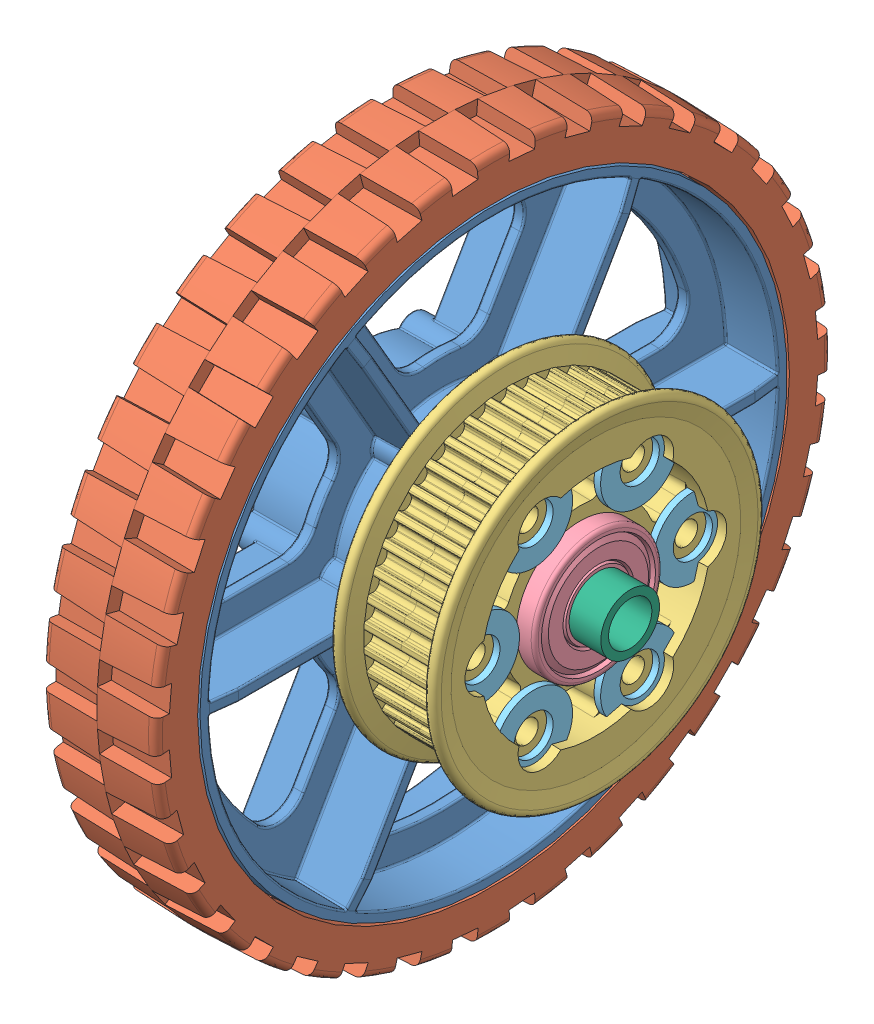
SolidWorks assembly 6 HiGrip with bearings, pulleys and spacers_2, configuration Default. Lengths in mm.
Overall size (85.56 152.4 152.4).
15 component instances, 7 part files, 0 mates.
Components (placement in the parent):
- 6 HiGrip Wheel Assembly Rev II-1: 6 HiGrip Wheel Assembly Rev II [Default] at (83.7987 67.439 110.9939) size (34.93 152.4 152.4)
  - 6 wheel Rev 4-1: 6 wheel Rev 4 [Default] at (-52.6446 9.4231 21.378) size (34.93 132.08 132.08)
  - 6 wheel tread II-1: 6 wheel tread II [Default] at (-65.3446 9.4231 21.378) x (0 0 -1) z (1 0 0) size (152.4 152.4 25.58)
- HalfPulley_42t5mm-1: HalfPulley_42t5mm [Default] at (47.6006 76.862 132.3719) x (1 0 0) z (0 -0.5 0.866025) size (13 74.23 74.23)
- HalfPulley_42t5mm-2: HalfPulley_42t5mm [Default] at (64.263 76.862 132.3719) x (-1 0 0) z (0 -0.499927 0.866067) size (13 74.23 74.23)
- Bearing_1614ZZ-1: Bearing_1614ZZ [Default] at (62.612 76.862 132.3719) x (0 -0.157148 -0.987575) z (-1 0 0) size (28.58 28.58 9.53)
- Bearing_1614ZZ-2: Bearing_1614ZZ [Default] at (15.2791 76.862 132.3719) x (0 0 -1) z (1 0 0) size (28.58 28.58 9.53)
- Washer_5-16-1: Washer_5-16 [Default] at (63.247 76.8605 108.5602) x (0 0.946124 0.323805) z (1 0 0) size (17.53 17.53 1.47)
- Washer_5-16-2: Washer_5-16 [Default] at (63.247 97.4833 120.4656) x (0 0.770474 -0.637472) z (1 0 0) size (17.53 17.53 1.47)
- Washer_5-16-3: Washer_5-16 [Default] at (63.247 56.2398 144.2799) x (0 0 -1) z (1 0 0) size (17.53 17.53 1.47)
- Washer_5-16-4: Washer_5-16 [Default] at (63.247 76.8625 156.1852) x (0 -0.95788 -0.287168) z (1 0 0) size (17.53 17.53 1.47)
- Washer_5-16-5: Washer_5-16 [Default] at (63.247 97.4843 144.2781) x (0 -0.653102 0.75727) z (1 0 0) size (17.53 17.53 1.47)
- Washer_5-16-6: Washer_5-16 [Default] at (63.247 56.2388 120.4674) x (0 -0.977348 -0.211637) z (1 0 0) size (17.53 17.53 1.47)
- Spacer_0.28x0.382-1: Spacer_0.28x0.382 [Default] at (74.4865 76.862 132.3719) x (0 -0.35357 0.935408) z (-1 0 0) size (13.16 13.16 7.11)
- Spacer_0.85x0.38-1: Spacer_0.85x0.38 [Default] at (-11.0734 76.862 132.3719) x (0 0 -1) z (1 0 0) size (19.05 19.05 21.59)
